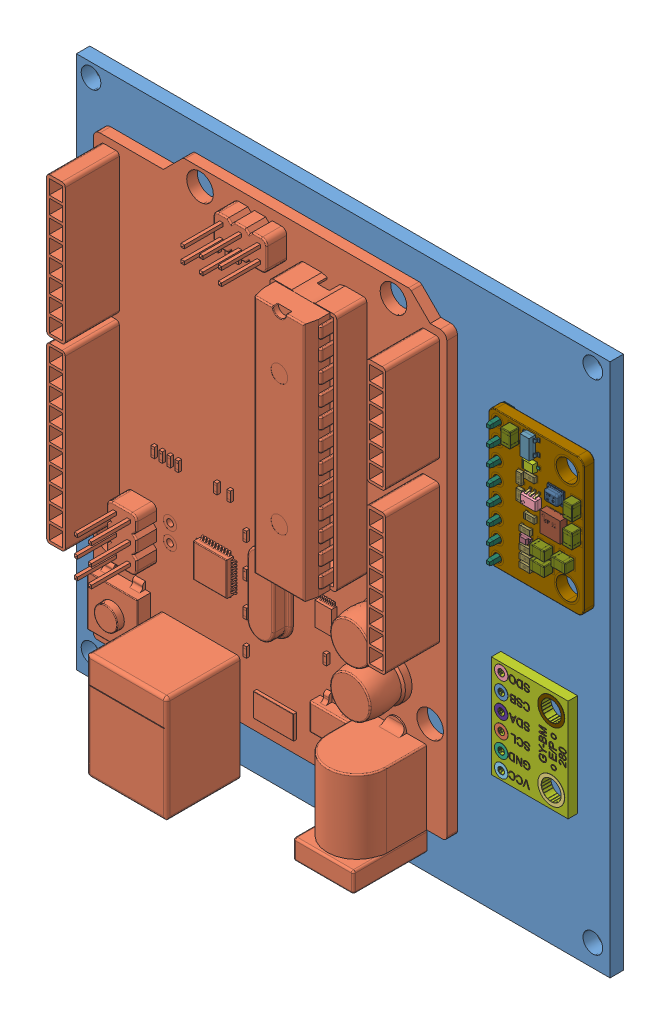
SolidWorks assembly OBC_4, configuration Default. Lengths in mm.
Overall size (80 80.42 20.96).
63 component instances, 29 part files, 0 mates.
Components (placement in the parent):
- Stack_plane_final-1: Stack_plane_final [Default] at (29.9812 39.7784 61.6823) size (80 80 2)
- arduino uno-1: arduino uno [Default] at (20.6017 39.8567 63.272) x (0 1 0) z (1 0 0) size (76.5 14.6 53)
- GY-91.STEP-1: GY-91.STEP [Default] at (57.713 76.0128 56.2619) x (1 0 0) z (0 -1 0) size (14.3 11.56 20.5)
  - TSSOP-6.STEP-1: TSSOP-6.STEP [Default] at (2.8163 9.9451 17.8096) x (-1 0 0) z (0 1 0) size (2.25 2.25 1.11)
    - User Library-TSSOP-6 (SOT-23-6 PITCH 0.65)_pin_TSSOP_tssop6_1.STEP-1: User Library-TSSOP-6 (SOT-23-6 PITCH 0.65)_pin_TSSOP_tssop6_1.STEP [Default] at (0.65 0.675 0) x (-1 0 0) z (0 1 0) size (0.3 0.82 0.45)
    - User Library-TSSOP-6 (SOT-23-6 PITCH 0.65)_pin_TSSOP_tssop6_1.STEP-2: User Library-TSSOP-6 (SOT-23-6 PITCH 0.65)_pin_TSSOP_tssop6_1.STEP [Default] at (0.65 -0.675 0) x (1 0 0) z (0 -1 0) size (0.3 0.82 0.45)
    - User Library-TSSOP-6 (SOT-23-6 PITCH 0.65)_pin_TSSOP_tssop6_1.STEP-3: User Library-TSSOP-6 (SOT-23-6 PITCH 0.65)_pin_TSSOP_tssop6_1.STEP [Default] at (-0.65 -0.675 0) x (1 0 0) z (0 -1 0) size (0.3 0.82 0.45)
    - User Library-TSSOP-6 (SOT-23-6 PITCH 0.65)_pin_TSSOP_tssop6_1.STEP-4: User Library-TSSOP-6 (SOT-23-6 PITCH 0.65)_pin_TSSOP_tssop6_1.STEP [Default] at (0 0.675 0) x (-1 0 0) z (0 1 0) size (0.3 0.82 0.45)
    - User Library-TSSOP-6 (SOT-23-6 PITCH 0.65)_pin_TSSOP_tssop6_1.STEP-5: User Library-TSSOP-6 (SOT-23-6 PITCH 0.65)_pin_TSSOP_tssop6_1.STEP [Default] at (-0.65 0.675 0) x (-1 0 0) z (0 1 0) size (0.3 0.82 0.45)
    - User Library-TSSOP-6 (SOT-23-6 PITCH 0.65)_pin_TSSOP_tssop6_1.STEP-6: User Library-TSSOP-6 (SOT-23-6 PITCH 0.65)_pin_TSSOP_tssop6_1.STEP [Default] at (0 -0.675 0) x (1 0 0) z (0 -1 0) size (0.3 0.82 0.45)
    - User Library-TSSOP-6 (SOT-23-6 PITCH 0.65)_body_TSSOP-6_TSSOP5_1.STEP-1: User Library-TSSOP-6 (SOT-23-6 PITCH 0.65)_body_TSSOP-6_TSSOP5_1.STEP [Default] at origin size (2.25 1.35 1)
  - Diode.STEP-1: Diode.STEP [Default] at (2.3136 9.1851 13.5607) x (0 0 1) z (0 1 0) size (1.25 2.5 0.7)
    - User Library-SMini2-F5-B_K.STEP-1: User Library-SMini2-F5-B_K.STEP [Default] at origin size (0.5 0.55 0.13)
    - User Library-SMini2-F5-B_A.STEP-1: User Library-SMini2-F5-B_A.STEP [Default] at origin size (0.35 0.55 0.13)
    - User Library-SMini2-F5-B_Diode.STEP-1: User Library-SMini2-F5-B_Diode.STEP [Default] at origin size (1.25 1.7 0.69)
    - User Library-SMini2-F5-B_Marker.STEP-1: User Library-SMini2-F5-B_Marker.STEP [Default] at origin size (1.13 0.07 0.01)
  - gy-91.STEP-1: gy-91.STEP [Default] at (-4.1995 7.585 9.2186) size (14.3 1.6 20.5)
  - BMP280___ _________.STEP-1: BMP280___ _________.STEP [Default] at (7.282 9.2051 14.714) x (-1 0 0) z (0 -1 0) size (2.5 2 0.97)
  - MPU9250.STEP-1: MPU9250.STEP [Default] at (6.0967 9.235 19.3741) x (-1 0 0) z (0 0 -1) size (3.02 1.05 3.02)
  - Res0603.STEP-1: Res0603.STEP [Default] at (0.7709 9.4101 18.2393) x (0 0 1) z (-1 0 0) size (1.6 0.45 0.8)
  - Res0603.STEP-2: Res0603.STEP [Default] at (0.7648 9.4101 15.9917) x (0 0 -1) z (1 0 0) size (1.6 0.45 0.8)
  - Res0603.STEP-3: Res0603.STEP [Default] at (2.312 9.4101 20.4364) size (1.6 0.45 0.8)
  - Res0603.STEP-4: Res0603.STEP [Default] at (1.6231 9.4101 26.0002) size (1.6 0.45 0.8)
  - Res0603.STEP-5: Res0603.STEP [Default] at (1.6278 9.4101 22.3827) size (1.6 0.45 0.8)
  - Res0603.STEP-6: Res0603.STEP [Default] at (2.2995 9.4101 15.1771) size (1.6 0.45 0.8)
  - Res0603.STEP-7: Res0603.STEP [Default] at (1.6136 9.4101 24.8159) size (1.6 0.45 0.8)
  - Res0603.STEP-8: Res0603.STEP [Default] at (1.6314 9.4101 27.1438) size (1.6 0.45 0.8)
  - LED0603.STEP-1: LED0603.STEP [Default] at (2.2297 9.1803 23.5734) x (0 0 1) z (0 1 0) size (0.72 1.65 0.68)
  - LDO SOT23.STEP-1: LDO SOT23.STEP [Default] at (2.3141 9.7351 10.8967) x (0 0 1) z (-1 0 0) size (3 1.1 2.5)
  - MalePinHeader.STEP-1: MalePinHeader.STEP [Default] at (-4.1268 5.0451 16.9269) size (2.54 11.54 2.54)
  - MalePinHeader.STEP-2: MalePinHeader.STEP [Default] at (-4.1071 5.0451 9.3011) size (2.54 11.54 2.54)
  - MalePinHeader.STEP-3: MalePinHeader.STEP [Default] at (-4.1137 5.0451 14.3787) size (2.54 11.54 2.54)
  - MalePinHeader.STEP-4: MalePinHeader.STEP [Default] at (-4.1149 5.0451 27.0667) size (2.54 11.54 2.54)
  - MalePinHeader.STEP-5: MalePinHeader.STEP [Default] at (-4.1277 5.0451 11.82) size (2.54 11.54 2.54)
  - MalePinHeader.STEP-6: MalePinHeader.STEP [Default] at (-4.1157 5.0451 24.5674) size (2.54 11.54 2.54)
  - MalePinHeader.STEP-7: MalePinHeader.STEP [Default] at (-4.1188 5.0451 22.0085) size (2.54 11.54 2.54)
  - MalePinHeader.STEP-8: MalePinHeader.STEP [Default] at (-4.1228 5.0451 19.4816) size (2.54 11.54 2.54)
  - Cap 0805.STEP-1: Cap 0805.STEP [Default] at (52.5692 21.2292 -81.079) x (0 0 -1) z (-1 0 0) size (2.29 1.46 1.49)
  - Cap 0805.STEP-2: Cap 0805.STEP [Default] at (101.2177 21.2292 66.9567) x (1 0 0) z (0 0 -1) size (2.29 1.46 1.49)
  - Cap 0805.STEP-3: Cap 0805.STEP [Default] at (43.25 21.2292 -85.9252) x (0 0 -1) z (-1 0 0) size (2.29 1.46 1.49)
  - Cap 0805.STEP-4: Cap 0805.STEP [Default] at (104.4136 21.2292 66.9514) x (1 0 0) z (0 0 -1) size (2.29 1.46 1.49)
  - Cap 0805.STEP-5: Cap 0805.STEP [Default] at (52.531 21.2292 -77.4673) x (0 0 -1) z (-1 0 0) size (2.29 1.46 1.49)
  - Cap 0805.STEP-6: Cap 0805.STEP [Default] at (101.2189 21.2292 68.9637) x (1 0 0) z (0 0 -1) size (2.29 1.46 1.49)
- P280, 6-PIN-Version v4.step-1: P280, 6-PIN-Version v4.step [Default] at (59.3565 26.3459 65.0982) x (0 1 0) z (0 0 -1) size (15.3 11.5 2.52)
  - PCB.step-1: PCB.step [Default] at origin size (15.3 11.5 1.62)
    - Komponente1.step-1: Komponente1.step [Default] at origin size (2 2 1.62)
    - Komponente2.step-1: Komponente2.step [Default] at origin size (4 4 1.62)
    - Komponente3.step-1: Komponente3.step [Default] at origin size (2 2 1.62)
    - Komponente4.step-1: Komponente4.step [Default] at origin size (2 2 1.62)
    - Komponente5.step-1: Komponente5.step [Default] at origin size (4 4 1.62)
    - Komponente6.step-1: Komponente6.step [Default] at origin size (2 2 1.62)
    - Komponente7.step-1: Komponente7.step [Default] at origin size (2 2 1.62)
    - Komponente8.step-1: Komponente8.step [Default] at origin size (2 2 1.62)
    - PCB-0.step-1: PCB-0.step [Default] at origin size (15.3 11.5 1.55)
  - Bauteile.step-1: Bauteile.step [Default] at origin size (8.8 7.18 0.94)
    - C0603.step-1: C0603.step [Default] at (9.1998 8.6998 1.5493) x (0 -1 0) z (0 0 -1) size (0.8 1.6 0.6)
    - R0603.step-1: R0603.step [Default] at (5.9383 -10.4268 1.548) x (-1 0 0) z (0 0 -1) size (0.8 1.6 0.3)
    - R0603.step-2: R0603.step [Default] at (1.9383 -10.4268 1.548) x (-1 0 0) z (0 0 -1) size (0.8 1.6 0.3)
    - R0603.step-3: R0603.step [Default] at (3.9383 -10.4268 1.548) x (-1 0 0) z (0 0 -1) size (0.8 1.6 0.3)
    - C0603.step-2: C0603.step [Default] at (-0.062 -10.4268 1.5473) x (-1 0 0) z (0 0 -1) size (0.8 1.6 0.6)
    - BME280.step-1: BME280.step [Default] at (2.5 12.9 -0.0401) x (-1 0 0) z (0 0 1) size (2.51 2.5 0.93)
    - R0603.step-4: R0603.step [Default] at (7.9383 -10.4268 1.548) x (-1 0 0) z (0 0 -1) size (0.8 1.6 0.3)
  - Beschriftung.step-1: Beschriftung.step [Default] at origin size (13.63 8.62 0.01)
